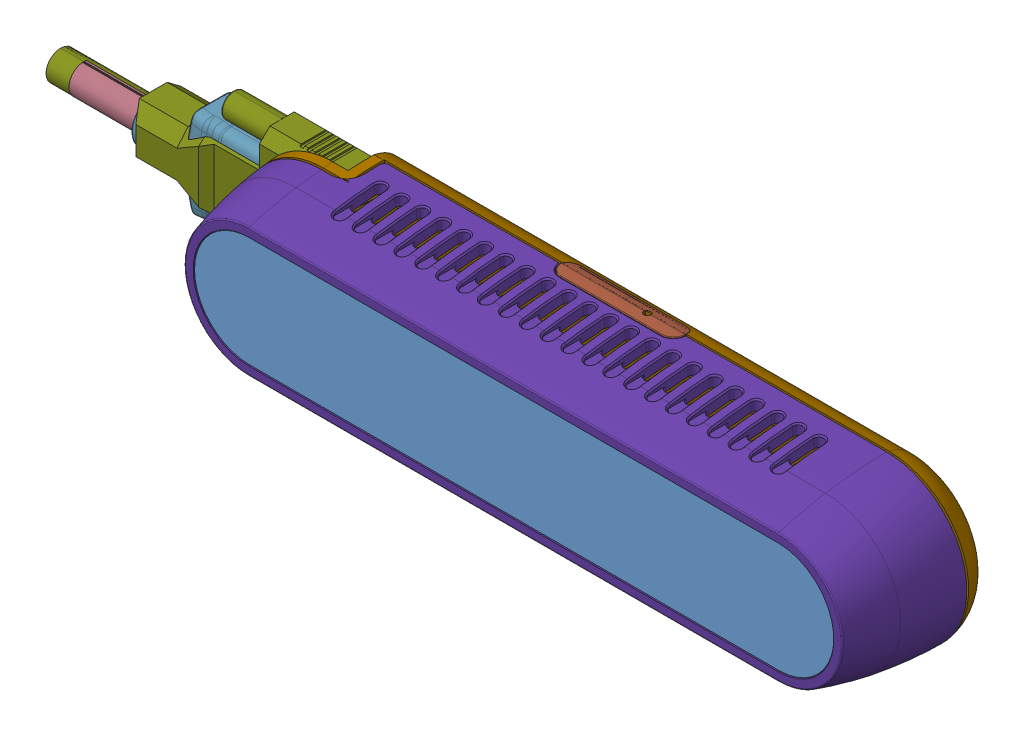
SolidWorks assembly Intel_RealSense_Depth_Camera_D415, configuration Default. Lengths in mm.
Overall size (130.85 23.53 20.08).
38 component instances, 23 part files, 0 mates.
Components (placement in the parent):
- Intel_RealSense_Depth_Camera_D415.STEP-1: Intel_RealSense_Depth_Camera_D415.STEP [Default] at origin size (130.85 23.53 20.08)
  - LENS_COVER_SUBASSY_ASRC_ASM.STEP-1: LENS_COVER_SUBASSY_ASRC_ASM.STEP [Default] at origin size (91.8 15.8 0.7)
    - LENS_COVER_ASRC.STEP-1: LENS_COVER_ASRC.STEP [Default] at origin size (91.8 15.8 0.55)
    - MASK_LENS_COVER_ASRC.STEP-1: MASK_LENS_COVER_ASRC.STEP [Default] at origin size (91.8 15.8 0.03)
    - ADHESIVE_LENS_COVER_ASRC.STEP-1: ADHESIVE_LENS_COVER_ASRC.STEP [Default] at origin size (91.2 15.2 0.13)
  - FOAM_ISOLATION_W_CARRIER_ASRC_ASM.STEP-1: FOAM_ISOLATION_W_CARRIER_ASRC_ASM.STEP [Default] at origin size (85.1 11.4 0.58)
    - DS5_0390_FOAM_FRONT.STEP-1: DS5_0390_FOAM_FRONT.STEP [Default] at origin size (85.1 11.4 0.53)
    - DS5_0390_ADHESIVE.STEP-1: DS5_0390_ADHESIVE.STEP [Default] at (0 0 -0.2) size (85.1 11.4 0.05)
  - CAMERA_MOD_DS5_ASRC_ASM.STEP-1: CAMERA_MOD_DS5_ASRC_ASM.STEP [Default] at (13.5 0 -6.04) x (1 0 0) z (0 -1 0) size (83.7 4.7 10)
    - IDC-DS-0601_ASRC_SW0001_1_ASM.STEP-1: IDC-DS-0601_ASRC_SW0001_1_ASM.STEP [Default] at origin size (83.7 4.7 10)
      - IDC-DS-0601_ASRC_SW0001_1_1.STEP-1: IDC-DS-0601_ASRC_SW0001_1_1.STEP [Default] at origin size (83.7 4.7 10)
  - LABEL_ASRC_CAMERA_MODULE_ASM.STEP-1: LABEL_ASRC_CAMERA_MODULE_ASM.STEP [Default] at origin size (82.7 9 0.55)
    - DS5_0390_LABEL_FRONT_MODULE.STEP-1: DS5_0390_LABEL_FRONT_MODULE.STEP [Default] at origin size (82.7 9 0.55)
    - DS5_0390_LABEL_FRONT_ADHESIVE.STEP-1: DS5_0390_LABEL_FRONT_ADHESIVE.STEP [Default] at origin size (82.7 9 0.03)
  - REAR_COVER_SUBASSY_ASRC_ASM.STEP-1: REAR_COVER_SUBASSY_ASRC_ASM.STEP [Default] at origin size (99.28 23.01 10.39)
    - REAR_COVER_ALUMINUM_ASRC.STEP-1: REAR_COVER_ALUMINUM_ASRC.STEP [Default] at origin size (99.28 23.01 10.39)
    - MAGNET.STEP-1: MAGNET.STEP [Default] at (-7.25 8.4 -15.54) x (-1 0 0) z (0 1 0) size (1.6 1.6 1.6)
    - MAGNET.STEP-2: MAGNET.STEP [Default] at (7.25 8.4 -15.54) x (-1 0 0) z (0 1 0) size (1.6 1.6 1.6)
  - AUX_COVER_SUBASSY_ASRC_ASM.STEP-1: AUX_COVER_SUBASSY_ASRC_ASM.STEP [Default] at origin size (17.9 3.6 3.42)
    - AUX_COVER_ALUMINUM_ASRC.STEP-1: AUX_COVER_ALUMINUM_ASRC.STEP [Default] at origin size (17.9 3.6 3.42)
    - PIN_STEEL_ZINC_PLATED.STEP-1: PIN_STEEL_ZINC_PLATED.STEP [Default] at (-7.25 10 -15.54) x (1 0 0) z (0 -1 0) size (1.6 1.6 1.6)
    - PIN_STEEL_ZINC_PLATED.STEP-2: PIN_STEEL_ZINC_PLATED.STEP [Default] at (7.25 10 -15.54) x (1 0 0) z (0 -1 0) size (1.6 1.6 1.6)
  - USB_TYPE-C_PLUG_-1_ASM.STEP-1: USB_TYPE-C_PLUG_-1_ASM.STEP [Default] at (-36.1 0 -15.875) x (0 -1 0) z (1 0 0) size (13.06 6.7 48.1)
    - USB_TYPE-C_PLUG_-1_1_ASM.STEP-1: USB_TYPE-C_PLUG_-1_1_ASM.STEP [Default] at origin size (13.06 6.7 48.1)
      - BOSS-EXTRUDE3.STEP-1: BOSS-EXTRUDE3.STEP [Default] at origin size (4.2 4.2 10)
      - FILLET11.STEP-1: FILLET11.STEP [Default] at origin size (13.06 6.7 31.5)
      - BOSS-EXTRUDE4.STEP-1: BOSS-EXTRUDE4.STEP [Default] at origin size (8.3 2.45 6.6)
  - LOCKING_CTYPE_USB_ASM.STEP-1: LOCKING_CTYPE_USB_ASM.STEP [Default] at (-36.15 0 -15.92) size (51.45 18.5 8)
    - LOCKING_C_TYPE_USB.STEP-1: LOCKING_C_TYPE_USB.STEP [Default] at origin size (48.3 18.5 8)
    - BOSS-EXTRUDE4.STEP-1: BOSS-EXTRUDE4.STEP [Default] at (6.65 -0.005 -0.005) x (0 -1 0) z (-1 0 0) size (8.3 2.45 6.6)
  - FRONT_COVER_ALUMINUM_ASRC.STEP-1: FRONT_COVER_ALUMINUM_ASRC.STEP [Default] at origin size (98.75 23.53 15.66)
  - HEATSINK_ASRC.STEP-1: HEATSINK_ASRC.STEP [Default] at origin size (94.31 20.8 12.15)
  - BRACKET_CAMERA_MODULE_ASRC.STEP-1: BRACKET_CAMERA_MODULE_ASRC.STEP [Default] at (5.175 0.35 -6.01) x (-1 0 0) z (0 1 0) size (21 5.77 15.8)
  - BRACKET_B2B_CONN_SUPPORT_ASRC.STEP-1: BRACKET_B2B_CONN_SUPPORT_ASRC.STEP [Default] at (5.2 -5.1 -0.87) size (14.5 6.47 1.64)
  - SCREW_TORX_M1-6_X_4L.STEP-1: SCREW_TORX_M1-6_X_4L.STEP [Default] at (-0.375 6.95 -7.86) size (3.2 3.2 5.3)
  - SCREW_TORX_M1-6_X_4L.STEP-2: SCREW_TORX_M1-6_X_4L.STEP [Default] at (10.725 6.95 -7.86) size (3.2 3.2 5.3)
  - SCREW_TORX_M2_X_5L.STEP-1: SCREW_TORX_M2_X_5L.STEP [Default] at (-39.8 0 -12.04) x (-1 0 0) z (0 0 -1) size (4 4 5)
  - BARCODE.STEP-1: BARCODE.STEP [Default] at (0 -9.728 -1.7983) x (-1 0 0) z (0 -0.968461 0.249165) size (70 5.5 0.09)
